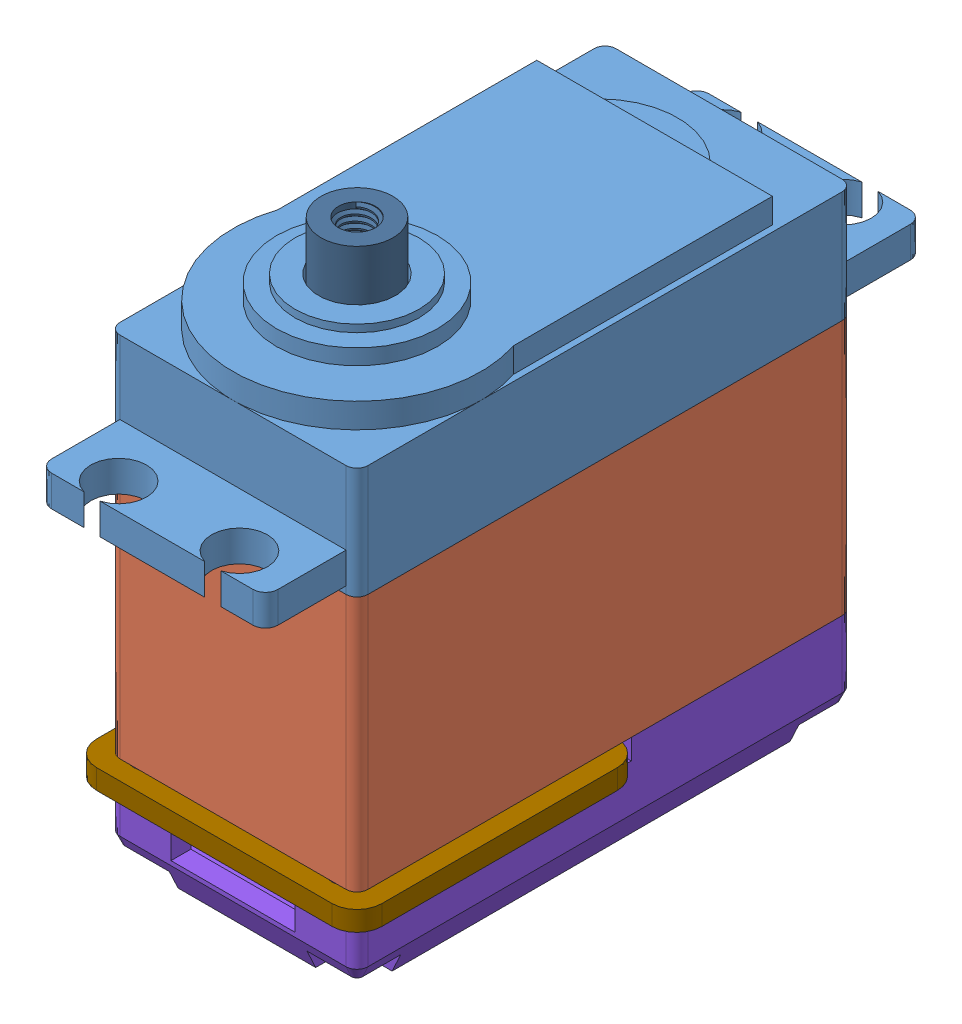
SolidWorks assembly asm, configuration Default. Lengths in mm.
Overall size (24.86 45.2 53).
14 component instances, 14 part files, 37 mates.
Components (placement in the parent):
- front_lid-1: front_lid [Default] at (26.2286 29.7028 32.7391) x (-1 0 0) z (0 0 -1) size (20 12.85 53)
- cover-1: cover [Default] at (26.2286 9.1028 32.7391) size (20 30.7 40)
- brushed_dc_motor-1: brushed_dc_motor [Default] at (26.2286 5.1028 22.1191) size (17 29.15 17)
- washer-1: washer [Default] at (26.2286 31.9028 42.7391) x (-0.926476 0 0.376355) z (-0.376355 0 -0.926476) size (10.7 2.4 10.7)
- gear_shaft-1: gear_shaft [Default] at (26.2286 11.0028 42.7391) x (-0.730663 0 -0.682739) z (0.682739 0 -0.730663) size (6.15 25.3 6.15)
- magnet-1: magnet [Default] at (26.2286 11.0028 42.7391) x (-0.213301 0 0.976987) z (-0.976987 0 -0.213301) size (4 1.95 4)
- shaft_support-1: shaft_support [Default] at (26.2286 28.1028 43.1891) x (1 0 0) z (0 0 -1) size (16.8 16.57 13.4)
- back_lid-2: back_lid [Default] at (26.2286 7.4528 32.7391) x (-1 0 0) z (0 0 -1) size (20 7.8 40)
- encoder-1: encoder [Default] at (26.2286 7.4528 42.7391) size (23 3.2 23)
- pot_gear-1: pot_gear [Default] at (26.2286 32.7028 42.7391) x (0.730663 0 0.682739) z (-0.682739 0 0.730663) size (17.6 14.7 17.57)
- mid_top_gear-1: mid_top_gear [Default] at (26.2286 35.9028 31.3391) x (0.380081 0 0.924953) z (0.924953 0 -0.380081) size (14.98 5.4 14.98)
- motor_top_gear-1: motor_top_gear [Default] at (26.2286 35.6028 22.1191) x (0.702122 0 -0.712056) z (0.712056 0 0.702122) size (14.98 7.3 14.98)
- mid_bottom_gear-1: mid_bottom_gear [Default] at (26.2286 30.7028 31.3391) x (0.963253 0 0.268595) z (-0.268595 0 0.963253) size (15.75 2.8 15.74)
- motor_gear-1: motor_gear [Default] at (26.2286 29.6028 22.1191) x (-0.718873 0 -0.695141) z (0.695141 0 -0.718873) size (3.25 2.3 3.22)
Mates (geometry in assembly coordinates):
- Coincident6: coincident anti-aligned: plane of cover-1 through (35.3486 29.7028 13.6191) normal (0 1 0); plane of front_lid-1 through (17.1086 29.7028 51.8591) normal (0 -1 0)
- Coincident8: coincident anti-aligned: plane of cover-1 through (26.2286 31.9028 42.7391) normal (0 1 0); plane of washer-1 through (26.2286 31.9028 42.7391) normal (0 -1 0)
- Concentric2: concentric aligned: cylinder of cover-1 through (26.2286 34.1528 42.7391) axis (0 -1 0) radius 3.4; cylinder of washer-1 through (26.2286 34.3028 42.7391) axis (0 -1 0) radius 3.4
- Coincident37: coincident anti-aligned: plane of cover-1 through (26.2286 28.1028 32.7391) normal (0 -1 0); plane of brushed_dc_motor-1 through (26.2286 28.1028 22.1191) normal (0 1 0)
- Concentric8: concentric anti-aligned: cylinder of cover-1 through (26.2286 18.1028 22.1191) axis (0 1 0) radius 8.5; cylinder of brushed_dc_motor-1 through (26.2286 28.1028 22.1191) axis (0 -1 0) radius 8.5
- Coincident42: coincident anti-aligned: plane of front_lid-1 through (17.1086 29.7028 51.8591) normal (0 -1 0); plane of cover-1 through (35.3486 29.7028 13.6191) normal (0 1 0)
- Coincident43: coincident aligned: plane of front_lid-1 through (16.2286 38.7028 51.8591) normal (-1 0 0); plane of cover-1 through (16.2286 29.7028 13.6191) normal (-1 0 0)
- Coincident44: coincident aligned: plane of front_lid-1 through (35.3486 38.7028 52.7391) normal (0 0 1); plane of cover-1 through (17.1086 29.7028 52.7391) normal (0 0 1)
- Coincident48: coincident anti-aligned: plane of cover-1 through (26.2286 28.1028 32.7391) normal (0 -1 0); plane of shaft_support-1 through (26.2286 28.1028 43.1891) normal (0 1 0)
- Coincident49: coincident anti-aligned: plane of cover-1 through (21.1036 24.5028 37.7391) normal (0 0 1); plane of shaft_support-1 through (21.1036 26.6028 37.7391) normal (0 0 -1)
- Coincident50: coincident anti-aligned: plane of cover-1 through (31.3536 24.5028 51.1391) normal (-1 0 0); plane of shaft_support-1 through (31.3536 26.6028 48.6391) normal (1 0 0)
- Coincident72: coincident anti-aligned: plane of cover-1 through (35.3486 9.1028 13.6191) normal (0 -1 0); plane of new_back_lid_v2-2 through (17.1086 9.1028 13.6191) normal (0 1 0)
- Coincident73: coincident aligned: plane of cover-1 through (36.2286 29.7028 13.6191) normal (1 0 0); plane of new_back_lid_v2-2 through (36.2286 3.7028 13.6191) normal (1 0 0)
- Coincident74: coincident aligned: plane of cover-1 through (17.1086 29.7028 12.7391) normal (0 0 -1); plane of new_back_lid_v2-2 through (35.3486 3.7028 12.7391) normal (0 0 -1)
- Concentric10: concentric aligned: circle of new_back_lid_v2-2; circle of encoder-1
- Coincident76: coincident anti-aligned: plane of new_back_lid_v2-2 through (17.1086 7.4528 13.6191) normal (0 1 0); plane of encoder-1 through (26.2286 7.4528 42.7391) normal (0 -1 0)
- Parallel2: parallel aligned: plane of new_back_lid_v2-2 through (16.2286 3.7028 13.6191) normal (-1 0 0); plane of encoder-1 through (14.7286 9.0528 31.2391) normal (-1 0 0)
- Parallel3: parallel anti-aligned: line of cover-1 through (17.1086 9.1028 51.8591) axis (0 0 -1); line of brushed_dc_motor-1 through (21.3786 2.7528 20.1191) axis (0 0 1)
- Concentric13: concentric aligned: cylinder of washer-1 through (26.2286 34.3028 42.7391) axis (0 -1 0) radius 3.4; cylinder of gear_shaft-1 through (26.2286 31.7528 42.7391) axis (0 -1 0) radius 1.8
- Concentric14: concentric aligned: cylinder of gear_shaft-1 through (26.2286 12.9528 42.7391) axis (0 -1 0) radius 2.15; cylinder of magnet-1 through (26.2286 12.9528 42.7391) axis (0 -1 0) radius 2
- Coincident84: coincident anti-aligned: plane of gear_shaft-1 through (26.2286 12.9528 42.7391) normal (0 -1 0); plane of magnet-1 through (26.2286 12.9528 42.7391) normal (0 1 0)
- Concentric15: concentric aligned: cylinder of washer-1 through (26.2286 34.3028 42.7391) axis (0 -1 0) radius 5.35; cylinder of pot_gear-1 through (26.2286 34.3028 42.7391) axis (0 -1 0) radius 5
- Coincident85: coincident anti-aligned: plane of washer-1 through (26.2286 34.3028 42.7391) normal (0 1 0); plane of pot_gear-1 through (26.2286 34.3028 42.7391) normal (0 -1 0)
- Coincident86: coincident anti-aligned: plane of gear_shaft-1 through (26.2286 36.3028 42.7391) normal (0 1 0); plane of pot_gear-1 through (26.2286 36.3028 42.7391) normal (0 -1 0)
- Parallel4: parallel anti-aligned: line of gear_shaft-1 through (25.908 36.3028 44.5103) axis (0.682739 0 -0.730663); line of pot_gear-1 through (28.1882 36.3028 42.1067) axis (-0.682739 0 0.730663)
- Concentric16: concentric aligned: cylinder of cover-1 through (26.2286 39.8028 31.3391) axis (0 -1 0) radius 0.8; cylinder of mid_top_gear-1 through (26.2286 37.9028 31.3391) axis (0 -1 0) radius 0.8
- Coincident87: coincident anti-aligned: plane of pot_gear-1 through (26.2286 35.9028 42.7391) normal (0 1 0); plane of mid_top_gear-1 through (26.2286 35.9028 31.3391) normal (0 -1 0)
- GearMate1: gear = 16.8 : 5.2 mm: circle of top_gear-1; circle of pot_gear-1
- Concentric17: concentric anti-aligned: cylinder of cover-1 through (26.2286 39.8028 22.1191) axis (0 -1 0) radius 0.8; cylinder of motor_top_gear-1 through (26.2286 31.1028 22.1191) axis (0 1 0) radius 0.8
- Coincident88: coincident anti-aligned: plane of cover-1 through (26.2286 34.5028 22.1191) normal (0 1 0); plane of motor_top_gear-1 through (26.2286 34.5028 22.1191) normal (0 -1 0)
- GearMate2: gear = 3.6 : 14.4 mm: circle of mid_top_gear-1; circle of motor_top_gear-1
- Concentric19: concentric anti-aligned: cylinder of cover-1 through (26.2286 39.8028 31.3391) axis (0 -1 0) radius 0.8; cylinder of mid_bottom_gear-1 through (26.2286 29.7028 31.3391) axis (0 1 0) radius 0.8
- Coincident89: coincident anti-aligned: plane of cover-1 through (35.3486 29.7028 13.6191) normal (0 1 0); plane of mid_bottom_gear-1 through (26.2286 29.7028 31.3391) normal (0 -1 0)
- GearMate3: gear = 14.4 : 3.6 mm: circle of mid_bottom_gear-1; circle of motor_top_gear-1
- Concentric21: concentric anti-aligned: cylinder of brushed_dc_motor-1 through (26.2286 31.9028 22.1191) axis (0 -1 0) radius 0.75; cylinder of motor_gear-1 through (26.2286 29.6028 22.1191) axis (0 1 0) radius 0.75
- Coincident90: coincident aligned: plane of brushed_dc_motor-1 through (26.2286 31.9028 22.1191) normal (0 1 0); plane of motor_gear-1 through (26.2286 31.9028 22.1191) normal (0 1 0)
- GearMate5: gear = 2.75 : 15.25 mm: circle of mid_bottom_gear-1; circle of motor_gear-1
